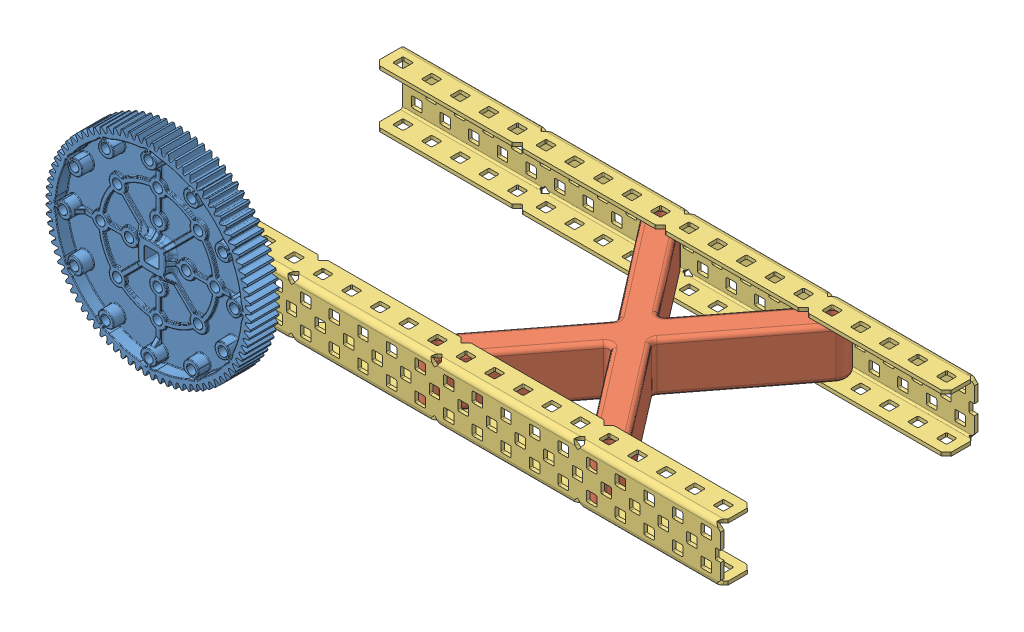
SolidWorks assembly RearArm_BottomBar, configuration Default. Lengths in mm.
Overall size (286.79 90.98 127).
4 component instances, 3 part files, 9 mates.
Components (placement in the parent):
- 84T High Strength Gear (276-3438)-1: 84T High Strength Gear (276-3438) [Default] at (-17.4079 64.2311 194.2288) size (90.98 90.98 12.7)
- ArmXBrace-1: ArmXBrace [Default] at (128.6421 53.1059 130.7288) x (0 0 1) z (-1 0 0) size (111.86 22.25 88.94)
- 1x2x1x20 Aluminum C-Channel-1: 1x2x1x20 Aluminum C-Channel [Default] at (192.1421 64.2311 187.8788) size (254 25.41 13.97)
- 1x2x1x20 Aluminum C-Channel-2: 1x2x1x20 Aluminum C-Channel [Default] at (192.1421 64.2311 73.5788) x (1 0 0) z (0 0 -1) size (254 25.41 13.97)
Mates (geometry in assembly coordinates):
- Concentric8: concentric aligned: cylinder of 84T High Strength Gear (276-3438)-1 through (-4.7079 64.2311 187.8788) axis (0 0 1) radius 2.1; circle of 1x2x1x20 Aluminum C-Channel-1
- Coincident9: coincident anti-aligned: plane of 84T High Strength Gear (276-3438)-1 through (-17.4079 109.7394 187.8788) normal (0 0 -1); plane of 1x2x1x20 Aluminum C-Channel-1 through (-29.6079 42.3108 187.8788) normal (0 0 1)
- Concentric9: concentric aligned: cylinder of 84T High Strength Gear (276-3438)-1 through (20.6921 64.2311 187.8788) axis (0 0 1) radius 2.1; circle of 1x2x1x20 Aluminum C-Channel-1
- Concentric10: concentric anti-aligned: cylinder of ArmXBrace-1 through (90.5421 75.3563 180.2588) axis (0 -1 0) radius 2.25; circle of 1x2x1x20 Aluminum C-Channel-1
- Coincident10: coincident anti-aligned: plane of ArmXBrace-1 through (128.6421 75.3563 130.7288) normal (0 1 0); plane of 1x2x1x20 Aluminum C-Channel-1 through (-29.6079 75.3563 220.2374) normal (0 -1 0)
- Concentric11: concentric anti-aligned: cylinder of ArmXBrace-1 through (166.7421 75.3563 180.2588) axis (0 -1 0) radius 2.25; circle of 1x2x1x20 Aluminum C-Channel-1
- Concentric12: concentric aligned: cylinder of ArmXBrace-1 through (90.5421 75.3563 81.1988) axis (0 -1 0) radius 2.25; circle of 1x2x1x20 Aluminum C-Channel-2
- Coincident11: coincident anti-aligned: plane of ArmXBrace-1 through (128.6421 75.3563 130.7288) normal (0 1 0); plane of 1x2x1x20 Aluminum C-Channel-2 through (-29.6079 75.3563 85.0607) normal (0 -1 0)
- Concentric13: concentric aligned: cylinder of ArmXBrace-1 through (166.7421 75.3563 81.1988) axis (0 -1 0) radius 2.25; circle of 1x2x1x20 Aluminum C-Channel-2
